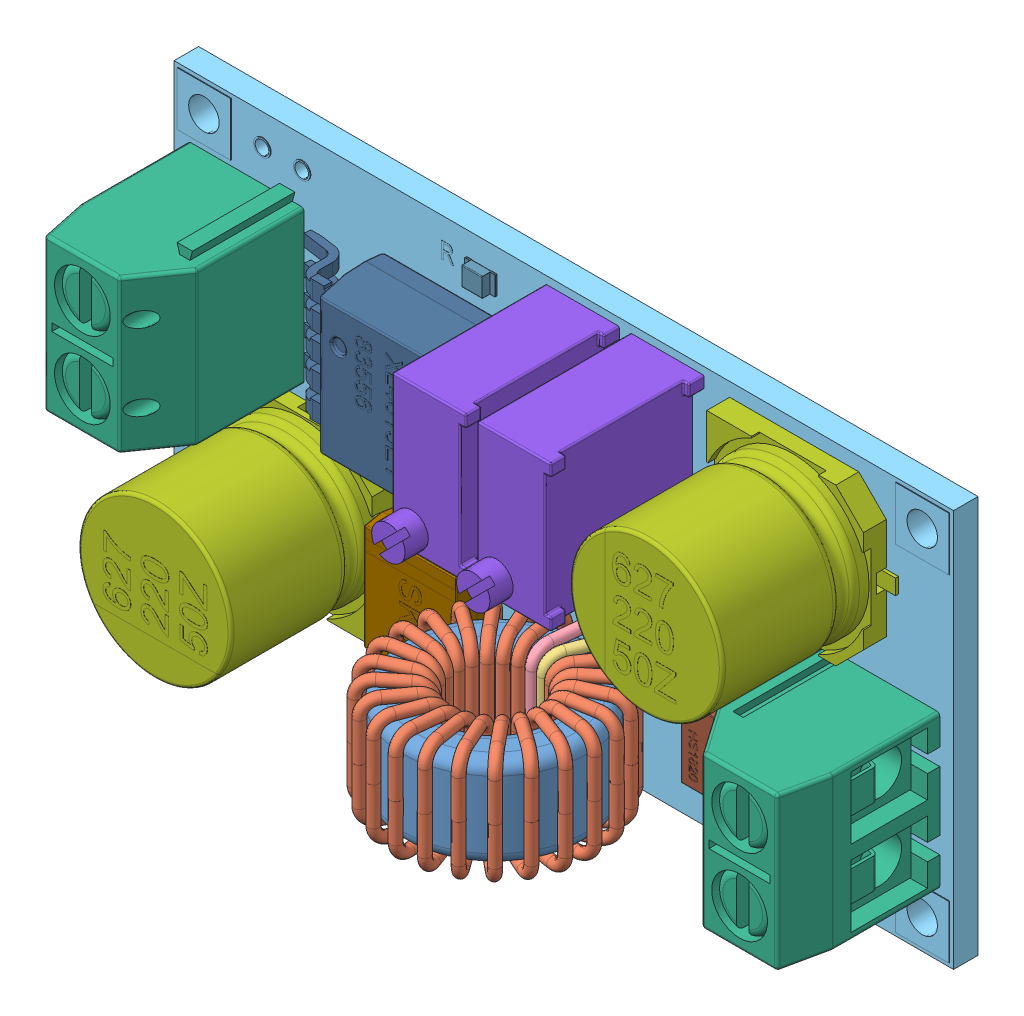
SolidWorks assembly XL4015 StepDown DC-DC 5A (CC-CV) v1, configuration Default. Lengths in mm.
Overall size (51 26 18.44).
42 component instances, 14 part files, 0 mates.
Components (placement in the parent):
- XL4015 StepDown DC-DC 5A (CC-CV) v1.step-1: XL4015 StepDown DC-DC 5A (CC-CV) v1.step [Default] at origin size (51 26 18.44)
  - Coil v9.step-1: Coil v9.step [Default] at (0 0 9) x (0 0 -1) z (0 -1 0) size (17.32 14.29 7.7)
    - Toro.step-1: Toro.step [Default] at (0.4 28 -5) size (13 12 6)
    - Spira.step-1: Spira.step [Default] at (0.4 28 -5) x (0.965926 0.258819 0) z (0 0 1) size (4.37 2.38 7.7)
    - Spira.step-2: Spira.step [Default] at (0.4 28 -5) x (0.866025 0.5 0) z (0 0 1) size (4.37 2.38 7.7)
    - Spira.step-3: Spira.step [Default] at (0.4 28 -5) x (0.707107 0.707107 0) z (0 0 1) size (4.37 2.38 7.7)
    - Spira.step-4: Spira.step [Default] at (0.4 28 -5) x (0.5 0.866025 0) z (0 0 1) size (4.37 2.38 7.7)
    - Spira.step-5: Spira.step [Default] at (0.4 28 -5) x (0.258819 0.965926 0) z (0 0 1) size (4.37 2.38 7.7)
    - Spira.step-6: Spira.step [Default] at (0.4 28 -5) x (0 1 0) z (0 0 1) size (4.37 2.38 7.7)
    - Spira.step-7: Spira.step [Default] at (0.4 28 -5) x (-0.258819 0.965926 0) z (0 0 1) size (4.37 2.38 7.7)
    - Spira.step-8: Spira.step [Default] at (0.4 28 -5) x (-0.5 0.866025 0) z (0 0 1) size (4.37 2.38 7.7)
    - Spira.step-9: Spira.step [Default] at (0.4 28 -5) x (-0.707107 0.707107 0) z (0 0 1) size (4.37 2.38 7.7)
    - Spira.step-10: Spira.step [Default] at (0.4 28 -5) x (-0.866025 0.5 0) z (0 0 1) size (4.37 2.38 7.7)
    - Spira.step-11: Spira.step [Default] at (0.4 28 -5) x (-0.965926 0.258819 0) z (0 0 1) size (4.37 2.38 7.7)
    - Spira.step-12: Spira.step [Default] at (0.4 28 -5) x (-1 0 0) z (0 0 1) size (4.37 2.38 7.7)
    - Spira.step-13: Spira.step [Default] at (0.4 28 -5) x (-0.965926 -0.258819 0) z (0 0 1) size (4.37 2.38 7.7)
    - Spira.step-14: Spira.step [Default] at (0.4 28 -5) x (-0.866025 -0.5 0) z (0 0 1) size (4.37 2.38 7.7)
    - Spira.step-15: Spira.step [Default] at (0.4 28 -5) x (-0.707107 -0.707107 0) z (0 0 1) size (4.37 2.38 7.7)
    - Spira.step-16: Spira.step [Default] at (0.4 28 -5) x (-0.5 -0.866025 0) z (0 0 1) size (4.37 2.38 7.7)
    - Spira.step-17: Spira.step [Default] at (0.4 28 -5) x (-0.258819 -0.965926 0) z (0 0 1) size (4.37 2.38 7.7)
    - Spira.step-18: Spira.step [Default] at (0.4 28 -5) x (0 -1 0) z (0 0 1) size (4.37 2.38 7.7)
    - Spira.step-19: Spira.step [Default] at (0.4 28 -5) x (0.258819 -0.965926 0) z (0 0 1) size (4.37 2.38 7.7)
    - Spira.step-20: Spira.step [Default] at (0.4 28 -5) x (0.5 -0.866025 0) z (0 0 1) size (4.37 2.38 7.7)
    - Spira.step-21: Spira.step [Default] at (0.4 28 -5) x (0.707107 -0.707107 0) z (0 0 1) size (4.37 2.38 7.7)
    - Spira.step-22: Spira.step [Default] at (0.4 28 -5) x (0.866025 -0.5 0) z (0 0 1) size (4.37 2.38 7.7)
    - SpiraCodA.step-1: SpiraCodA.step [Default] at (0.4015 27.9945 -5) x (1 0.000874 0) z (0 0 1) size (7.52 2.39 7.7)
    - SpiraCpdB.step-1: SpiraCpdB.step [Default] at (0.399 27.9963 -5) x (0.966079 -0.258245 0) z (0 0 1) size (7.28 3.27 7.7)
  - Basetta.step-1: Basetta.step [Default] at origin size (51 26 1.7)
  - DG301-5.0-02 v1.step-1: DG301-5.0-02 v1.step [Default] at (4 19.4 1.6) x (0 -1 0) z (0 0 1) size (10.6 7.6 14.3)
  - DG301-5.0-02 v1.step-2: DG301-5.0-02 v1.step [Default] at (47 6.6 1.6) x (0 1 0) z (0 0 1) size (10.6 7.6 14.3)
  - CAPACITOR 10x10 SMD v1.step-1: CAPACITOR 10x10 SMD v1.step [Default] at (9.325 5.925 1.6) x (1 0 0) z (0 -1 0) size (10.25 10.61 11.85)
  - CAPACITOR 10x10 SMD v1.step-2: CAPACITOR 10x10 SMD v1.step [Default] at (41.475 19.975 1.6) x (0 -1 0) z (-1 0 0) size (10.25 10.61 11.85)
  - Trimpot 3296W v1.step-1: Trimpot 3296W v1.step [Default] at (26.715 20.735 1.6) x (0 -1 0) z (0 0 1) size (9.56 4.83 14.15)
  - Trimpot 3296W v1.step-2: Trimpot 3296W v1.step [Default] at (32.265 20.735 1.6) x (0 -1 0) z (0 0 1) size (9.56 4.83 14.15)
  - DO-214AB v1.step-1: DO-214AB v1.step [Default] at (18.1 1.725 1.6) x (0 1 0) z (0 0 1) size (8.15 6.25 2.66)
  - XL4015 TO263-5-1 v1.step-1: XL4015 TO263-5-1 v1.step [Default] at (18.4666 17.0892 1.5654) x (0 -1 0) z (-0.006883 0 0.999976) size (9.82 14.6 4.22)
  - LM358 SOIC08 v1.step-1: LM358 SOIC08 v1.step [Default] at (37 6 1.55) x (0 -1 0) z (0 0 1) size (5 6.17 2.02)
  - UPC78L08T-E1-AZ.step-1: UPC78L08T-E1-AZ.step [Default] at (31.81 12.82 1.6) x (0 1 0) z (0 0 1) size (4.36 4 1.51)
  - SC-59A v1.step-1: SC-59A v1.step [Default] at (36.8 13.75 1.6) x (0 -1 0) z (0 0 1) size (3.1 3 1.45)
  - LED v1.step-1: LED v1.step [Default] at (44.84 1.625 1.62) x (0 -1 0) z (-1 0 0) size (1.27 0.67 2.02)
  - LED v1.step-2: LED v1.step [Default] at (39.84 1.625 1.62) x (0 -1 0) z (-1 0 0) size (1.27 0.67 2.02)
  - LED v1.step-3: LED v1.step [Default] at (20.16 23.875 1.62) x (0 -1 0) z (-1 0 0) size (1.27 0.67 2.02)
